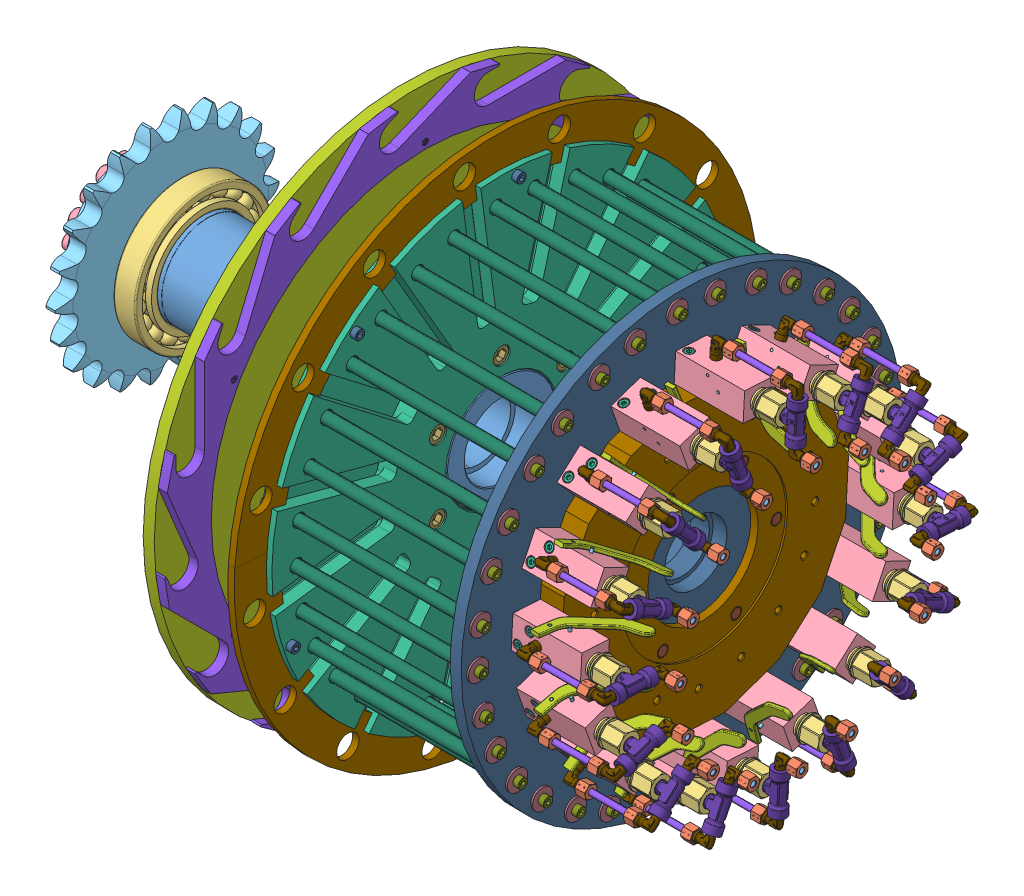
SolidWorks assembly assieme parte rotante, configuration Default. Lengths in mm. (continued)
Components (placement in the parent): (continued)
- AssiemeValvola-7: AssiemeValvola [Default] at (515.3257 -134.8578 488.6421) x (0 0.901303 -0.433189) z (0 -0.433189 -0.901303) size (90.26 138.63 38)
  - RaccordoT-1: RaccordoT [Default] at origin size (43 29.75 16.5)
  - Raccordo a L-1: Raccordo a L [Default] at (-30 0 0) x (0 -1 0) z (0 0 -1) size (28.34 25.51 14.01)
    - 1809_06_10_01-1: 1809_06_10_01 [Default] at origin size (22.49 23 10)
    - 1809_06_10_02-1: 1809_06_10_02 [Default] at origin size (6.5 8.5 8.5)
    - 1809_06_10_03-1: 1809_06_10_03 [Default] at origin size (11.02 15.01 14.01)
  - Raccordo a L-2: Raccordo a L [Default] at (30 0 0) x (0 1 0) z (0 0 -1) size (28.34 25.51 14.01)
    - 1809_06_10_01-1: 1809_06_10_01 [Default] at origin size (22.49 23 10)
    - 1809_06_10_02-1: 1809_06_10_02 [Default] at origin size (6.5 8.5 8.5)
    - 1809_06_10_03-1: 1809_06_10_03 [Default] at origin size (11.02 15.01 14.01)
  - TappoChiusura-1: TappoChiusura [Default] at (0 -32 0) x (0 -1 0) z (0 0 1) size (38.28 26.74 26.74)
  - CorpoValvola-1: CorpoValvola [Default] at (-15 -115.2824 0) size (30 75 34)
  - Raccordo a L-3: Raccordo a L [Default] at (-30 -88.2824 0) x (0 1 0) z (0 0 1) size (28.34 25.51 14.01)
    - 1809_06_10_01-1: 1809_06_10_01 [Default] at origin size (22.49 23 10)
    - 1809_06_10_02-1: 1809_06_10_02 [Default] at origin size (6.5 8.5 8.5)
    - 1809_06_10_03-1: 1809_06_10_03 [Default] at origin size (11.02 15.01 14.01)
  - Spina_3x38-1: Spina_3x38 [Default] at (0 -68.2824 -21) x (-1 0 0) z (0 0 1) size (3 3 38)
  - Spina_3x38-2: Spina_3x38 [Default] at (-10 -80.2824 -21) x (0.996193 0.087174 0) z (0 0 1) size (3 3 38)
  - M5 40mm-3: M5 40mm [ISO 4762 M5 x 40 - 40N] at (-14.6 -108.7824 9) size (45 8.5 8.5)
  - M5 40mm-2: M5 40mm [ISO 4762 M5 x 40 - 40N] at (-14.6 -96.7824 -9) size (45 8.5 8.5)
  - LevaValvola-1: LevaValvola [Default] at (-24.507 -86.571 -17) x (0.996193 0.087174 0) z (0 0 1) size (77.55 60.2 4)
  - Tubo-1: Tubo [Default] at (-30 -15.9665 0) x (1 0 0) z (0 -1 0) size (6 6 56.4)
- AssiemeValvola-8: AssiemeValvola [Default] at (515.3257 -95.0129 541.6718) x (0 0.666921 -0.745128) z (0 -0.745128 -0.666921) size (90.26 138.63 38)
  - RaccordoT-1: RaccordoT [Default] at origin size (43 29.75 16.5)
  - Raccordo a L-1: Raccordo a L [Default] at (-30 0 0) x (0 -1 0) z (0 0 -1) size (28.34 25.51 14.01)
    - 1809_06_10_01-1: 1809_06_10_01 [Default] at origin size (22.49 23 10)
    - 1809_06_10_02-1: 1809_06_10_02 [Default] at origin size (6.5 8.5 8.5)
    - 1809_06_10_03-1: 1809_06_10_03 [Default] at origin size (11.02 15.01 14.01)
  - Raccordo a L-2: Raccordo a L [Default] at (30 0 0) x (0 1 0) z (0 0 -1) size (28.34 25.51 14.01)
    - 1809_06_10_01-1: 1809_06_10_01 [Default] at origin size (22.49 23 10)
    - 1809_06_10_02-1: 1809_06_10_02 [Default] at origin size (6.5 8.5 8.5)
    - 1809_06_10_03-1: 1809_06_10_03 [Default] at origin size (11.02 15.01 14.01)
  - TappoChiusura-1: TappoChiusura [Default] at (0 -32 0) x (0 -1 0) z (0 0 1) size (38.28 26.74 26.74)
  - CorpoValvola-1: CorpoValvola [Default] at (-15 -115.2824 0) size (30 75 34)
  - Raccordo a L-3: Raccordo a L [Default] at (-30 -88.2824 0) x (0 1 0) z (0 0 1) size (28.34 25.51 14.01)
    - 1809_06_10_01-1: 1809_06_10_01 [Default] at origin size (22.49 23 10)
    - 1809_06_10_02-1: 1809_06_10_02 [Default] at origin size (6.5 8.5 8.5)
    - 1809_06_10_03-1: 1809_06_10_03 [Default] at origin size (11.02 15.01 14.01)
  - Spina_3x38-1: Spina_3x38 [Default] at (0 -68.2824 -21) x (-1 0 0) z (0 0 1) size (3 3 38)
  - Spina_3x38-2: Spina_3x38 [Default] at (-10 -80.2824 -21) x (0.996193 0.087174 0) z (0 0 1) size (3 3 38)
  - M5 40mm-3: M5 40mm [ISO 4762 M5 x 40 - 40N] at (-14.6 -108.7824 9) size (45 8.5 8.5)
  - M5 40mm-2: M5 40mm [ISO 4762 M5 x 40 - 40N] at (-14.6 -96.7824 -9) size (45 8.5 8.5)
  - LevaValvola-1: LevaValvola [Default] at (-24.507 -86.571 -17) x (0.996193 0.087174 0) z (0 0 1) size (77.55 60.2 4)
  - Tubo-1: Tubo [Default] at (-30 -15.9665 0) x (1 0 0) z (0 -1 0) size (6 6 56.4)
- AssiemeValvola-9: AssiemeValvola [Default] at (515.3257 -37.9074 575.4168) x (0 0.331007 -0.943628) z (0 -0.943628 -0.331007) size (90.26 138.63 38)
  - RaccordoT-1: RaccordoT [Default] at origin size (43 29.75 16.5)
  - Raccordo a L-1: Raccordo a L [Default] at (-30 0 0) x (0 -1 0) z (0 0 -1) size (28.34 25.51 14.01)
    - 1809_06_10_01-1: 1809_06_10_01 [Default] at origin size (22.49 23 10)
    - 1809_06_10_02-1: 1809_06_10_02 [Default] at origin size (6.5 8.5 8.5)
    - 1809_06_10_03-1: 1809_06_10_03 [Default] at origin size (11.02 15.01 14.01)
  - Raccordo a L-2: Raccordo a L [Default] at (30 0 0) x (0 1 0) z (0 0 -1) size (28.34 25.51 14.01)
    - 1809_06_10_01-1: 1809_06_10_01 [Default] at origin size (22.49 23 10)
    - 1809_06_10_02-1: 1809_06_10_02 [Default] at origin size (6.5 8.5 8.5)
    - 1809_06_10_03-1: 1809_06_10_03 [Default] at origin size (11.02 15.01 14.01)
  - TappoChiusura-1: TappoChiusura [Default] at (0 -32 0) x (0 -1 0) z (0 0 1) size (38.28 26.74 26.74)
  - CorpoValvola-1: CorpoValvola [Default] at (-15 -115.2824 0) size (30 75 34)
  - Raccordo a L-3: Raccordo a L [Default] at (-30 -88.2824 0) x (0 1 0) z (0 0 1) size (28.34 25.51 14.01)
    - 1809_06_10_01-1: 1809_06_10_01 [Default] at origin size (22.49 23 10)
    - 1809_06_10_02-1: 1809_06_10_02 [Default] at origin size (6.5 8.5 8.5)
    - 1809_06_10_03-1: 1809_06_10_03 [Default] at origin size (11.02 15.01 14.01)
  - Spina_3x38-1: Spina_3x38 [Default] at (0 -68.2824 -21) x (-1 0 0) z (0 0 1) size (3 3 38)
  - Spina_3x38-2: Spina_3x38 [Default] at (-10 -80.2824 -21) x (0.996193 0.087174 0) z (0 0 1) size (3 3 38)
  - M5 40mm-3: M5 40mm [ISO 4762 M5 x 40 - 40N] at (-14.6 -108.7824 9) size (45 8.5 8.5)
  - M5 40mm-2: M5 40mm [ISO 4762 M5 x 40 - 40N] at (-14.6 -96.7824 -9) size (45 8.5 8.5)
  - LevaValvola-1: LevaValvola [Default] at (-24.507 -86.571 -17) x (0.996193 0.087174 0) z (0 0 1) size (77.55 60.2 4)
  - Tubo-1: Tubo [Default] at (-30 -15.9665 0) x (1 0 0) z (0 -1 0) size (6 6 56.4)
- AssiemeValvola-10: AssiemeValvola [Default] at (515.3257 27.7648 584.7399) x (0 -0.055301 -0.99847) z (0 -0.99847 0.055301) size (90.26 138.63 38)
  - RaccordoT-1: RaccordoT [Default] at origin size (43 29.75 16.5)
  - Raccordo a L-1: Raccordo a L [Default] at (-30 0 0) x (0 -1 0) z (0 0 -1) size (28.34 25.51 14.01)
    - 1809_06_10_01-1: 1809_06_10_01 [Default] at origin size (22.49 23 10)
    - 1809_06_10_02-1: 1809_06_10_02 [Default] at origin size (6.5 8.5 8.5)
    - 1809_06_10_03-1: 1809_06_10_03 [Default] at origin size (11.02 15.01 14.01)
  - Raccordo a L-2: Raccordo a L [Default] at (30 0 0) x (0 1 0) z (0 0 -1) size (28.34 25.51 14.01)
    - 1809_06_10_01-1: 1809_06_10_01 [Default] at origin size (22.49 23 10)
    - 1809_06_10_02-1: 1809_06_10_02 [Default] at origin size (6.5 8.5 8.5)
    - 1809_06_10_03-1: 1809_06_10_03 [Default] at origin size (11.02 15.01 14.01)
  - TappoChiusura-1: TappoChiusura [Default] at (0 -32 0) x (0 -1 0) z (0 0 1) size (38.28 26.74 26.74)
  - CorpoValvola-1: CorpoValvola [Default] at (-15 -115.2824 0) size (30 75 34)
  - Raccordo a L-3: Raccordo a L [Default] at (-30 -88.2824 0) x (0 1 0) z (0 0 1) size (28.34 25.51 14.01)
    - 1809_06_10_01-1: 1809_06_10_01 [Default] at origin size (22.49 23 10)
    - 1809_06_10_02-1: 1809_06_10_02 [Default] at origin size (6.5 8.5 8.5)
    - 1809_06_10_03-1: 1809_06_10_03 [Default] at origin size (11.02 15.01 14.01)
  - Spina_3x38-1: Spina_3x38 [Default] at (0 -68.2824 -21) x (-1 0 0) z (0 0 1) size (3 3 38)
  - Spina_3x38-2: Spina_3x38 [Default] at (-10 -80.2824 -21) x (0.996193 0.087174 0) z (0 0 1) size (3 3 38)
  - M5 40mm-3: M5 40mm [ISO 4762 M5 x 40 - 40N] at (-14.6 -108.7824 9) size (45 8.5 8.5)
  - M5 40mm-2: M5 40mm [ISO 4762 M5 x 40 - 40N] at (-14.6 -96.7824 -9) size (45 8.5 8.5)
  - LevaValvola-1: LevaValvola [Default] at (-24.507 -86.571 -17) x (0.996193 0.087174 0) z (0 0 1) size (77.55 60.2 4)
  - Tubo-1: Tubo [Default] at (-30 -15.9665 0) x (1 0 0) z (0 -1 0) size (6 6 56.4)
- AssiemeValvola-11: AssiemeValvola [Default] at (515.3257 92.0058 568.2215) x (0 -0.433189 -0.901303) z (0 -0.901303 0.433189) size (90.26 138.63 38)
  - RaccordoT-1: RaccordoT [Default] at origin size (43 29.75 16.5)
  - Raccordo a L-1: Raccordo a L [Default] at (-30 0 0) x (0 -1 0) z (0 0 -1) size (28.34 25.51 14.01)
    - 1809_06_10_01-1: 1809_06_10_01 [Default] at origin size (22.49 23 10)
    - 1809_06_10_02-1: 1809_06_10_02 [Default] at origin size (6.5 8.5 8.5)
    - 1809_06_10_03-1: 1809_06_10_03 [Default] at origin size (11.02 15.01 14.01)
  - Raccordo a L-2: Raccordo a L [Default] at (30 0 0) x (0 1 0) z (0 0 -1) size (28.34 25.51 14.01)
    - 1809_06_10_01-1: 1809_06_10_01 [Default] at origin size (22.49 23 10)
    - 1809_06_10_02-1: 1809_06_10_02 [Default] at origin size (6.5 8.5 8.5)
    - 1809_06_10_03-1: 1809_06_10_03 [Default] at origin size (11.02 15.01 14.01)
  - TappoChiusura-1: TappoChiusura [Default] at (0 -32 0) x (0 -1 0) z (0 0 1) size (38.28 26.74 26.74)
  - CorpoValvola-1: CorpoValvola [Default] at (-15 -115.2824 0) size (30 75 34)
  - Raccordo a L-3: Raccordo a L [Default] at (-30 -88.2824 0) x (0 1 0) z (0 0 1) size (28.34 25.51 14.01)
    - 1809_06_10_01-1: 1809_06_10_01 [Default] at origin size (22.49 23 10)
    - 1809_06_10_02-1: 1809_06_10_02 [Default] at origin size (6.5 8.5 8.5)
    - 1809_06_10_03-1: 1809_06_10_03 [Default] at origin size (11.02 15.01 14.01)
  - Spina_3x38-1: Spina_3x38 [Default] at (0 -68.2824 -21) x (-1 0 0) z (0 0 1) size (3 3 38)
  - Spina_3x38-2: Spina_3x38 [Default] at (-10 -80.2824 -21) x (0.996193 0.087174 0) z (0 0 1) size (3 3 38)
  - M5 40mm-3: M5 40mm [ISO 4762 M5 x 40 - 40N] at (-14.6 -108.7824 9) size (45 8.5 8.5)
  - M5 40mm-2: M5 40mm [ISO 4762 M5 x 40 - 40N] at (-14.6 -96.7824 -9) size (45 8.5 8.5)
  - LevaValvola-1: LevaValvola [Default] at (-24.507 -86.571 -17) x (0.996193 0.087174 0) z (0 0 1) size (77.55 60.2 4)
  - Tubo-1: Tubo [Default] at (-30 -15.9665 0) x (1 0 0) z (0 -1 0) size (6 6 56.4)
- AssiemeValvola-12: AssiemeValvola [Default] at (515.3257 145.0355 528.3766) x (0 -0.745128 -0.666921) z (0 -0.666921 0.745128) size (90.26 138.63 38)
  - RaccordoT-1: RaccordoT [Default] at origin size (43 29.75 16.5)
  - Raccordo a L-1: Raccordo a L [Default] at (-30 0 0) x (0 -1 0) z (0 0 -1) size (28.34 25.51 14.01)
    - 1809_06_10_01-1: 1809_06_10_01 [Default] at origin size (22.49 23 10)
    - 1809_06_10_02-1: 1809_06_10_02 [Default] at origin size (6.5 8.5 8.5)
    - 1809_06_10_03-1: 1809_06_10_03 [Default] at origin size (11.02 15.01 14.01)
  - Raccordo a L-2: Raccordo a L [Default] at (30 0 0) x (0 1 0) z (0 0 -1) size (28.34 25.51 14.01)
    - 1809_06_10_01-1: 1809_06_10_01 [Default] at origin size (22.49 23 10)
    - 1809_06_10_02-1: 1809_06_10_02 [Default] at origin size (6.5 8.5 8.5)
    - 1809_06_10_03-1: 1809_06_10_03 [Default] at origin size (11.02 15.01 14.01)
  - TappoChiusura-1: TappoChiusura [Default] at (0 -32 0) x (0 -1 0) z (0 0 1) size (38.28 26.74 26.74)
  - CorpoValvola-1: CorpoValvola [Default] at (-15 -115.2824 0) size (30 75 34)
  - Raccordo a L-3: Raccordo a L [Default] at (-30 -88.2824 0) x (0 1 0) z (0 0 1) size (28.34 25.51 14.01)
    - 1809_06_10_01-1: 1809_06_10_01 [Default] at origin size (22.49 23 10)
    - 1809_06_10_02-1: 1809_06_10_02 [Default] at origin size (6.5 8.5 8.5)
    - 1809_06_10_03-1: 1809_06_10_03 [Default] at origin size (11.02 15.01 14.01)
  - Spina_3x38-1: Spina_3x38 [Default] at (0 -68.2824 -21) x (-1 0 0) z (0 0 1) size (3 3 38)
  - Spina_3x38-2: Spina_3x38 [Default] at (-10 -80.2824 -21) x (0.996193 0.087174 0) z (0 0 1) size (3 3 38)
  - M5 40mm-3: M5 40mm [ISO 4762 M5 x 40 - 40N] at (-14.6 -108.7824 9) size (45 8.5 8.5)
  - M5 40mm-2: M5 40mm [ISO 4762 M5 x 40 - 40N] at (-14.6 -96.7824 -9) size (45 8.5 8.5)
  - LevaValvola-1: LevaValvola [Default] at (-24.507 -86.571 -17) x (0.996193 0.087174 0) z (0 0 1) size (77.55 60.2 4)
  - Tubo-1: Tubo [Default] at (-30 -15.9665 0) x (1 0 0) z (0 -1 0) size (6 6 56.4)
- AssiemeValvola-13: AssiemeValvola [Default] at (515.3257 178.7805 471.2711) x (0 -0.943628 -0.331007) z (0 -0.331007 0.943628) size (90.26 138.63 38)
  - RaccordoT-1: RaccordoT [Default] at origin size (43 29.75 16.5)
  - Raccordo a L-1: Raccordo a L [Default] at (-30 0 0) x (0 -1 0) z (0 0 -1) size (28.34 25.51 14.01)
    - 1809_06_10_01-1: 1809_06_10_01 [Default] at origin size (22.49 23 10)
    - 1809_06_10_02-1: 1809_06_10_02 [Default] at origin size (6.5 8.5 8.5)
    - 1809_06_10_03-1: 1809_06_10_03 [Default] at origin size (11.02 15.01 14.01)
  - Raccordo a L-2: Raccordo a L [Default] at (30 0 0) x (0 1 0) z (0 0 -1) size (28.34 25.51 14.01)
    - 1809_06_10_01-1: 1809_06_10_01 [Default] at origin size (22.49 23 10)
    - 1809_06_10_02-1: 1809_06_10_02 [Default] at origin size (6.5 8.5 8.5)
    - 1809_06_10_03-1: 1809_06_10_03 [Default] at origin size (11.02 15.01 14.01)
  - TappoChiusura-1: TappoChiusura [Default] at (0 -32 0) x (0 -1 0) z (0 0 1) size (38.28 26.74 26.74)
  - CorpoValvola-1: CorpoValvola [Default] at (-15 -115.2824 0) size (30 75 34)
  - Raccordo a L-3: Raccordo a L [Default] at (-30 -88.2824 0) x (0 1 0) z (0 0 1) size (28.34 25.51 14.01)
    - 1809_06_10_01-1: 1809_06_10_01 [Default] at origin size (22.49 23 10)
    - 1809_06_10_02-1: 1809_06_10_02 [Default] at origin size (6.5 8.5 8.5)
    - 1809_06_10_03-1: 1809_06_10_03 [Default] at origin size (11.02 15.01 14.01)
  - Spina_3x38-1: Spina_3x38 [Default] at (0 -68.2824 -21) x (-1 0 0) z (0 0 1) size (3 3 38)
  - Spina_3x38-2: Spina_3x38 [Default] at (-10 -80.2824 -21) x (0.996193 0.087174 0) z (0 0 1) size (3 3 38)
  - M5 40mm-3: M5 40mm [ISO 4762 M5 x 40 - 40N] at (-14.6 -108.7824 9) size (45 8.5 8.5)
  - M5 40mm-2: M5 40mm [ISO 4762 M5 x 40 - 40N] at (-14.6 -96.7824 -9) size (45 8.5 8.5)
  - LevaValvola-1: LevaValvola [Default] at (-24.507 -86.571 -17) x (0.996193 0.087174 0) z (0 0 1) size (77.55 60.2 4)
  - Tubo-1: Tubo [Default] at (-30 -15.9665 0) x (1 0 0) z (0 -1 0) size (6 6 56.4)
- AssiemeValvola-14: AssiemeValvola [Default] at (515.3257 188.1036 405.5989) x (0 -0.99847 0.055301) z (0 0.055301 0.99847) size (90.26 138.63 38)
  - RaccordoT-1: RaccordoT [Default] at origin size (43 29.75 16.5)
  - Raccordo a L-1: Raccordo a L [Default] at (-30 0 0) x (0 -1 0) z (0 0 -1) size (28.34 25.51 14.01)
    - 1809_06_10_01-1: 1809_06_10_01 [Default] at origin size (22.49 23 10)
    - 1809_06_10_02-1: 1809_06_10_02 [Default] at origin size (6.5 8.5 8.5)
    - 1809_06_10_03-1: 1809_06_10_03 [Default] at origin size (11.02 15.01 14.01)
  - Raccordo a L-2: Raccordo a L [Default] at (30 0 0) x (0 1 0) z (0 0 -1) size (28.34 25.51 14.01)
    - 1809_06_10_01-1: 1809_06_10_01 [Default] at origin size (22.49 23 10)
    - 1809_06_10_02-1: 1809_06_10_02 [Default] at origin size (6.5 8.5 8.5)
    - 1809_06_10_03-1: 1809_06_10_03 [Default] at origin size (11.02 15.01 14.01)
  - TappoChiusura-1: TappoChiusura [Default] at (0 -32 0) x (0 -1 0) z (0 0 1) size (38.28 26.74 26.74)
  - CorpoValvola-1: CorpoValvola [Default] at (-15 -115.2824 0) size (30 75 34)
  - Raccordo a L-3: Raccordo a L [Default] at (-30 -88.2824 0) x (0 1 0) z (0 0 1) size (28.34 25.51 14.01)
    - 1809_06_10_01-1: 1809_06_10_01 [Default] at origin size (22.49 23 10)
    - 1809_06_10_02-1: 1809_06_10_02 [Default] at origin size (6.5 8.5 8.5)
    - 1809_06_10_03-1: 1809_06_10_03 [Default] at origin size (11.02 15.01 14.01)
  - Spina_3x38-1: Spina_3x38 [Default] at (0 -68.2824 -21) x (-1 0 0) z (0 0 1) size (3 3 38)
  - Spina_3x38-2: Spina_3x38 [Default] at (-10 -80.2824 -21) x (0.996193 0.087174 0) z (0 0 1) size (3 3 38)
  - M5 40mm-3: M5 40mm [ISO 4762 M5 x 40 - 40N] at (-14.6 -108.7824 9) size (45 8.5 8.5)
  - M5 40mm-2: M5 40mm [ISO 4762 M5 x 40 - 40N] at (-14.6 -96.7824 -9) size (45 8.5 8.5)
  - LevaValvola-1: LevaValvola [Default] at (-24.507 -86.571 -17) x (0.996193 0.087174 0) z (0 0 1) size (77.55 60.2 4)
  - Tubo-1: Tubo [Default] at (-30 -15.9665 0) x (1 0 0) z (0 -1 0) size (6 6 56.4)
- AssiemeValvola-15: AssiemeValvola [Default] at (515.3257 171.5852 341.3579) x (0 -0.901303 0.433189) z (0 0.433189 0.901303) size (90.26 138.63 38)
  - RaccordoT-1: RaccordoT [Default] at origin size (43 29.75 16.5)
  - Raccordo a L-1: Raccordo a L [Default] at (-30 0 0) x (0 -1 0) z (0 0 -1) size (28.34 25.51 14.01)
    - 1809_06_10_01-1: 1809_06_10_01 [Default] at origin size (22.49 23 10)
    - 1809_06_10_02-1: 1809_06_10_02 [Default] at origin size (6.5 8.5 8.5)
    - 1809_06_10_03-1: 1809_06_10_03 [Default] at origin size (11.02 15.01 14.01)
  - Raccordo a L-2: Raccordo a L [Default] at (30 0 0) x (0 1 0) z (0 0 -1) size (28.34 25.51 14.01)
    - 1809_06_10_01-1: 1809_06_10_01 [Default] at origin size (22.49 23 10)
    - 1809_06_10_02-1: 1809_06_10_02 [Default] at origin size (6.5 8.5 8.5)
    - 1809_06_10_03-1: 1809_06_10_03 [Default] at origin size (11.02 15.01 14.01)
  - TappoChiusura-1: TappoChiusura [Default] at (0 -32 0) x (0 -1 0) z (0 0 1) size (38.28 26.74 26.74)
  - CorpoValvola-1: CorpoValvola [Default] at (-15 -115.2824 0) size (30 75 34)
  - Raccordo a L-3: Raccordo a L [Default] at (-30 -88.2824 0) x (0 1 0) z (0 0 1) size (28.34 25.51 14.01)
    - 1809_06_10_01-1: 1809_06_10_01 [Default] at origin size (22.49 23 10)
    - 1809_06_10_02-1: 1809_06_10_02 [Default] at origin size (6.5 8.5 8.5)
    - 1809_06_10_03-1: 1809_06_10_03 [Default] at origin size (11.02 15.01 14.01)
  - Spina_3x38-1: Spina_3x38 [Default] at (0 -68.2824 -21) x (-1 0 0) z (0 0 1) size (3 3 38)
  - Spina_3x38-2: Spina_3x38 [Default] at (-10 -80.2824 -21) x (0.996193 0.087174 0) z (0 0 1) size (3 3 38)
  - M5 40mm-3: M5 40mm [ISO 4762 M5 x 40 - 40N] at (-14.6 -108.7824 9) size (45 8.5 8.5)
  - M5 40mm-2: M5 40mm [ISO 4762 M5 x 40 - 40N] at (-14.6 -96.7824 -9) size (45 8.5 8.5)
  - LevaValvola-1: LevaValvola [Default] at (-24.507 -86.571 -17) x (0.996193 0.087174 0) z (0 0 1) size (77.55 60.2 4)
  - Tubo-1: Tubo [Default] at (-30 -15.9665 0) x (1 0 0) z (0 -1 0) size (6 6 56.4)
- AssiemeValvola-16: AssiemeValvola [Default] at (515.3257 131.7403 288.3282) x (0 -0.666921 0.745128) z (0 0.745128 0.666921) size (90.26 138.63 38)
  - RaccordoT-1: RaccordoT [Default] at origin size (43 29.75 16.5)
  - Raccordo a L-1: Raccordo a L [Default] at (-30 0 0) x (0 -1 0) z (0 0 -1) size (28.34 25.51 14.01)
    - 1809_06_10_01-1: 1809_06_10_01 [Default] at origin size (22.49 23 10)
    - 1809_06_10_02-1: 1809_06_10_02 [Default] at origin size (6.5 8.5 8.5)
    - 1809_06_10_03-1: 1809_06_10_03 [Default] at origin size (11.02 15.01 14.01)
  - Raccordo a L-2: Raccordo a L [Default] at (30 0 0) x (0 1 0) z (0 0 -1) size (28.34 25.51 14.01)
    - 1809_06_10_01-1: 1809_06_10_01 [Default] at origin size (22.49 23 10)
    - 1809_06_10_02-1: 1809_06_10_02 [Default] at origin size (6.5 8.5 8.5)
    - 1809_06_10_03-1: 1809_06_10_03 [Default] at origin size (11.02 15.01 14.01)
  - TappoChiusura-1: TappoChiusura [Default] at (0 -32 0) x (0 -1 0) z (0 0 1) size (38.28 26.74 26.74)
  - CorpoValvola-1: CorpoValvola [Default] at (-15 -115.2824 0) size (30 75 34)
  - Raccordo a L-3: Raccordo a L [Default] at (-30 -88.2824 0) x (0 1 0) z (0 0 1) size (28.34 25.51 14.01)
    - 1809_06_10_01-1: 1809_06_10_01 [Default] at origin size (22.49 23 10)
    - 1809_06_10_02-1: 1809_06_10_02 [Default] at origin size (6.5 8.5 8.5)
    - 1809_06_10_03-1: 1809_06_10_03 [Default] at origin size (11.02 15.01 14.01)
  - Spina_3x38-1: Spina_3x38 [Default] at (0 -68.2824 -21) x (-1 0 0) z (0 0 1) size (3 3 38)
  - Spina_3x38-2: Spina_3x38 [Default] at (-10 -80.2824 -21) x (0.996193 0.087174 0) z (0 0 1) size (3 3 38)
  - M5 40mm-3: M5 40mm [ISO 4762 M5 x 40 - 40N] at (-14.6 -108.7824 9) size (45 8.5 8.5)
  - M5 40mm-2: M5 40mm [ISO 4762 M5 x 40 - 40N] at (-14.6 -96.7824 -9) size (45 8.5 8.5)
  - LevaValvola-1: LevaValvola [Default] at (-24.507 -86.571 -17) x (0.996193 0.087174 0) z (0 0 1) size (77.55 60.2 4)
  - Tubo-1: Tubo [Default] at (-30 -15.9665 0) x (1 0 0) z (0 -1 0) size (6 6 56.4)
- Disco alimentazione guarnizione fi24.4-1: Disco alimentazione guarnizione fi24.4 [Default] at (198.0433 18.3637 415) x (0 0.065403 0.997859) z (-1 0 0) size (570 285 7.35)
- Disco alimentazione guarnizione fi24.4-2: Disco alimentazione guarnizione fi24.4 [Default] at (198.0433 18.3637 415) x (0 -0.065403 -0.997859) z (-1 0 0) size (570 285 7.35)
- m6 12mm-1: m6 12mm [ISO 4762 M6 x 12 - 12N] at (210.0433 200.6849 574.8914) x (-1 0 0) z (0 0.793353 -0.608761) size (18 10 10)
- m6 12mm-7: m6 12mm [ISO 4762 M6 x 12 - 12N] at (210.0433 260.3445 399.1397) x (-1 0 0) z (0 0.793353 -0.608761) size (18 10 10)
- m6 12mm-8: m6 12mm [ISO 4762 M6 x 12 - 12N] at (210.0433 96.3128 185.3694) x (-1 0 0) z (0 0.793353 -0.608761) size (18 10 10)
- m6 12mm-9: m6 12mm [ISO 4762 M6 x 12 - 12N] at (210.0433 -59.5854 644.6306) x (-1 0 0) z (0 -0.793353 -0.608761) size (18 10 10)
- m6 12mm-10: m6 12mm [ISO 4762 M6 x 12 - 12N] at (210.0433 -223.6171 430.8603) x (-1 0 0) z (0 -0.793353 -0.608761) size (18 10 10)
- m6 12mm-11: m6 12mm [ISO 4762 M6 x 12 - 12N] at (210.0433 -163.9575 255.1086) x (-1 0 0) z (0 0.793353 -0.608761) size (18 10 10)
Mates (geometry in assembly coordinates):
- Concentrico1: concentric anti-aligned: circle of albero rotazione piatti-1; circle of seger 100mm-1
- Coincidente1: coincident anti-aligned: plane of albero rotazione piatti-1 through (-143.4567 18.3637 415) normal (-1 0 0); plane of seger 100mm-1 through (-143.4567 18.3637 415) normal (1 0 0)
- Coincidente2: coincident aligned: plane of albero rotazione piatti-1 through (60.413 18.3637 415) normal (0 1 0); plane of seger 100mm-1 through (-146.4567 18.3637 415) normal (0 1 0)
- Concentrico21: concentric aligned: cylinder of albero rotazione piatti-1 through (60.413 18.3637 415) axis (1 0 0) radius 50; cylinder of SKF - 6020 - 20,DE,NC,20_68-1 through (-152.0942 18.3637 415) axis (1 0 0) radius 50
- Coincidente3: coincident anti-aligned: plane of seger 100mm-1 through (-143.4567 18.3637 415) normal (1 0 0); plane of SKF - 6020 - 20,DE,NC,20_68-1 through (-143.4567 -33.4256 439.9823) normal (-1 0 0)
- Concentrico3: concentric aligned: cylinder of albero rotazione piatti-1 through (60.413 18.3637 415) axis (1 0 0) radius 47.5; cylinder of calettatore d95-1 through (-199.9572 18.3637 415) axis (1 0 0) radius 47.5
- Concentrico4: concentric anti-aligned: cylinder of calettatore d95-1 through (-196.9572 18.3637 415) axis (1 0 0) radius 67.5; cylinder of pulegia z =50-1 through (-170.9572 18.3637 415) axis (-1 0 0) radius 67.5
- Coincidente4: coincident anti-aligned: plane of calettatore d95-1 through (-170.9572 84.9137 415) normal (1 0 0); plane of pulegia z =50-1 through (-170.9572 18.3637 415) normal (-1 0 0)
- Coincidente5: coincident anti-aligned: plane of albero rotazione piatti-1 through (-155.9567 18.3637 415) normal (-1 0 0); plane of pulegia z =50-1 through (-155.9567 18.3637 415) normal (1 0 0)
- Coincidente6: coincident aligned: plane of calettatore d95-1 through (-184.9572 18.3637 415) normal (0 1 0); plane of pulegia z =50-1 through (-173.9167 18.3637 415) normal (0 1 0)
- Coincidente7: coincident aligned: plane of albero rotazione piatti-1 through (60.413 18.3637 415) normal (0 1 0); plane of calettatore d95-1 through (-184.9572 18.3637 415) normal (0 1 0)
- Concentrico5: concentric aligned: cylinder of albero rotazione piatti-1 through (60.413 18.3637 415) axis (1 0 0) radius 49.75; cylinder of SKF - 6020 - 20,DE,NC,20_68-2 through (41.4058 18.3637 415) axis (1 0 0) radius 50
- Coincidente8: coincident anti-aligned: plane of albero rotazione piatti-1 through (74.0433 18.3637 415) normal (-1 0 0); plane of SKF - 6020 - 20,DE,NC,20_68-2 through (74.0433 -28.0673 437.2803) normal (1 0 0)
- Concentrico6: concentric aligned: cylinder of albero rotazione piatti-1 through (60.413 18.3637 415) axis (1 0 0) radius 60; cylinder of Disco supporto montaggio e Colonne-1 through (5.3377 18.3637 415) axis (1 0 0) radius 60
- Concentrico7: concentric aligned: cylinder of albero rotazione piatti-1 through (101.3656 98.3637 415) axis (1 0 0) radius 6.25; cylinder of Disco supporto montaggio e Colonne-1 through (204.0433 98.3637 415) axis (1 0 0) radius 9.25
- Coincidente9: coincident anti-aligned: plane of albero rotazione piatti-1 through (175.0433 18.3637 415) normal (1 0 0); plane of Disco supporto montaggio e Colonne-1 through (175.0433 18.3637 415) normal (-1 0 0)
- Concentrico8: concentric anti-aligned: cylinder of albero rotazione piatti-1 through (60.413 18.3637 415) axis (1 0 0) radius 60; cylinder of piatto rotante porta tappi-1 through (111.0433 18.3637 415) axis (-1 0 0) radius 60
- Concentrico9: concentric aligned: circle of albero rotazione piatti-1; circle of piatto rotante porta tappi-1
- Coincidente10: coincident anti-aligned: plane of albero rotazione piatti-1 through (119.0433 18.3637 415) normal (-1 0 0); plane of piatto rotante porta tappi-1 through (119.0433 18.3637 415) normal (1 0 0)
- Concentrico10: concentric aligned: cylinder of piatto rotante porta tappi-1 through (119.0433 18.3637 415) axis (-1 0 0) radius 233; cylinder of disco trasportatore tappi 31-1 through (121.0433 18.3637 415) axis (-1 0 0) radius 233
- Tangente2: tangent: cylinder of piatto rotante porta tappi-1 through (98.5243 -101.6363 622.8461) axis (1 0 0) radius 3.25; curve of disco trasportatore tappi 31-1
- Coincidente13: coincident anti-aligned: plane of piatto rotante porta tappi-1 through (111.0433 18.3637 415) normal (1 0 0); plane of disco trasportatore tappi 31-1 through (111.0433 18.3637 415) normal (-1 0 0)
- Concentrico11: concentric anti-aligned: cylinder of albero rotazione piatti-1 through (60.413 18.3637 415) axis (1 0 0) radius 40; cylinder of disco trascinato porta distributore vuoto-1 through (400.0433 18.3637 415) axis (-1 0 0) radius 30
- Concentrico12: concentric anti-aligned: cylinder of Disco supporto montaggio e Colonne-1 through (204.0433 -202.0247 450.2415) axis (1 0 0) radius 6; cylinder of disco trascinato porta distributore vuoto-1 through (417.0139 -202.0247 450.2415) axis (-1 0 0) radius 6
- Coincidente14: coincident anti-aligned: plane of Distributore Rotante-1 through (400.0433 18.3637 415) normal (-1 0 0); plane of disco trascinato porta distributore vuoto-1 through (400.0433 18.3637 415) normal (1 0 0)
- Concentrico13: concentric anti-aligned: circle of Distributore Rotante-1; circle of disco trascinato porta distributore vuoto-1
- Concentrico14: concentric anti-aligned: cylinder of Distributore Rotante-1 through (230.3377 18.3637 415) axis (1 0 0) radius 60; cylinder of disco trascinato porta distributore vuoto-1 through (415.0433 18.3637 415) axis (-1 0 0) radius 67.5
- Concentrico15: concentric anti-aligned: cylinder of disco trascinato porta distributore vuoto-1 through (388.0433 -53.0243 378.8925) axis (1 0 0) radius 6.25; cylinder of m12 35mm-1 through (344.2933 -53.0243 378.8925) axis (-1 0 0) radius 6
- Coincidente15: coincident anti-aligned: plane of disco trascinato porta distributore vuoto-1 through (388.0433 18.3637 415) normal (-1 0 0); plane of m12 35mm-1 through (388.0433 -45.2301 383.3925) normal (1 0 0)
- Parallelo1: parallel anti-aligned: plane of m12 35mm-1 through (382.0433 -47.9668 381.8125) normal (0 -1 0)
- Concentrico16: concentric aligned: cylinder of Disco supporto montaggio e Colonne-1 through (204.0433 -21.6363 345.718) axis (1 0 0) radius 9.25; cylinder of m12 90mm-3 through (234.7933 -21.6363 345.718) axis (1 0 0) radius 6
- Coincidente17: coincident anti-aligned: plane of Disco supporto montaggio e Colonne-1 through (191.0433 -27.049 342.593) normal (1 0 0); plane of m12 90mm-3 through (191.0433 -29.4305 341.218) normal (-1 0 0)
- Parallelo2: parallel aligned: plane of m12 35mm-1 through (382.0433 -47.9668 381.8125) normal (0 -1 0); plane of m12 90mm-3 through (197.0433 -16.5788 348.6379) normal (0 -1 0)
- Concentrico171: concentric anti-aligned: cylinder of piatto rotante porta tappi-1 through (98.5243 -101.6363 207.1539) axis (1 0 0) radius 3.25; cylinder of rondella m6 22mm-1 through (64.1183 -101.6363 207.1539) axis (-1 0 0) radius 3.3
- Coincidente191: coincident anti-aligned: plane of piatto rotante porta tappi-1 through (99.0433 18.3637 415) normal (-1 0 0); plane of rondella m6 22mm-1 through (99.0433 -101.6363 210.4539) normal (1 0 0)
- Parallelo3: parallel anti-aligned: plane of rondella m6 22mm-1 through (99.0433 -101.6363 207.1539) normal (0 -1 0)
- Concentrico181: concentric aligned: cylinder of rondella m6 22mm-1 through (64.1183 -101.6363 207.1539) axis (-1 0 0) radius 3.3; cylinder of M6 20mm-1 through (59.2933 -101.6363 207.1539) axis (-1 0 0) radius 5
- Coincidente211: coincident anti-aligned: plane of rondella m6 22mm-1 through (97.0433 -101.6363 218.1539) normal (-1 0 0); plane of M6 20mm-1 through (97.0433 -97.3062 204.6539) normal (1 0 0)
- Parallelo4: parallel aligned: plane of m12 35mm-1 through (382.0433 -47.9668 381.8125) normal (0 -0.5 -0.866025); plane of M6 20mm-1 through (94.0433 -101.6363 210.0892) normal (0 -0.5 -0.866025)
- Concentrico19: concentric anti-aligned: cylinder of Disco supporto montaggio e Colonne-1 through (204.0433 70.1437 197.9013) axis (1 0 0) radius 6; cylinder of asta scorrimento carello-1 through (400.0433 70.1437 197.9013) axis (-1 0 0) radius 6
- Concentrico201: concentric aligned: cylinder of asta scorrimento carello-1 through (175.0433 70.1437 197.9013) axis (-1 0 0) radius 3.2; cylinder of rondella m6 22mm-7 through (140.1183 70.1437 197.9013) axis (-1 0 0) radius 3.3
- Coincidente231: coincident anti-aligned: plane of asta scorrimento carello-1 through (175.0433 70.1437 197.9013) normal (-1 0 0); plane of rondella m6 22mm-7 through (175.0433 70.1437 201.2013) normal (1 0 0)
- Concentrico211: concentric aligned: cylinder of rondella m6 22mm-7 through (140.1183 70.1437 197.9013) axis (-1 0 0) radius 3.3; cylinder of M6 16mm-1 through (135.2933 70.1437 197.9013) axis (-1 0 0) radius 5
- Coincidente241: coincident anti-aligned: plane of rondella m6 22mm-7 through (173.0433 70.1437 208.9013) normal (-1 0 0); plane of M6 16mm-1 through (173.0433 75.1437 197.9013) normal (1 0 0)
- Parallelo5: parallel aligned: plane of asta scorrimento carello-1 through (287.5433 70.1437 197.9013) normal (0 0 -1); plane of M6 16mm-1 through (170.0433 68.6761 200.4433) normal (0 0 -1)
- Parallelo9: parallel anti-aligned: plane of rondella m6 22mm-7 through (175.0433 70.1437 197.9013) normal (0 0 1); plane of M6 16mm-1 through (170.0433 68.6761 200.4433) normal (0 0 -1)
- Coincidente30: coincident anti-aligned: plane of Disco supporto montaggio e Colonne-1 through (175.0433 18.3637 415) normal (-1 0 0); plane of rondella m6 22mm-7 through (175.0433 70.1437 201.2013) normal (1 0 0)
- Coincidente31: coincident anti-aligned: plane of disco trascinato porta distributore vuoto-1 through (400.0433 18.3637 415) normal (1 0 0); plane of rondella m6 22mm-8 through (400.0433 70.1437 201.2013) normal (-1 0 0)
- Coincidente32: coincident anti-aligned: plane of Distributore Rotante-1 through (400.0433 40.5763 258.5322) normal (0 0.331007 -0.943628); plane of AssiemeValvola-1/CorpoValvola-1 through (400.0433 85.7114 274.3647) normal (0 -0.331007 0.943628)
- Coincidente33: coincident anti-aligned: plane of disco trascinato porta distributore vuoto-1 through (400.0433 18.3637 415) normal (1 0 0); plane of AssiemeValvola-1/CorpoValvola-1 through (400.0433 95.6416 246.0559) normal (-1 0 0)
- Concentrico22: concentric anti-aligned: cylinder of Distributore Rotante-1 through (412.5433 55.4365 309.3136) axis (0 0.331007 -0.943628) radius 3; cylinder of AssiemeValvola-1/CorpoValvola-1 through (412.5433 69.6697 268.7376) axis (0 -0.331007 0.943628) radius 3
- Concentrico23: concentric anti-aligned: cylinder of Disco supporto montaggio e Colonne-1 through (198.0433 18.3637 415) axis (-1 0 0) radius 235; cylinder of Disco alimentazione guarnizione fi24.4-2 through (191.0433 18.3637 415) axis (1 0 0) radius 235
- Concentrico24: concentric anti-aligned: cylinder of Disco supporto montaggio e Colonne-1 through (198.0433 18.3637 415) axis (-1 0 0) radius 235; cylinder of Disco alimentazione guarnizione fi24.4-1 through (191.0433 18.3637 415) axis (1 0 0) radius 235
- Coincidente34: coincident anti-aligned: plane of Disco alimentazione guarnizione fi24.4-1 through (191.0433 33.7334 649.4968) normal (0 -0.997859 0.065403); plane of Disco alimentazione guarnizione fi24.4-2 through (191.0433 37.0036 699.3898) normal (0 0.997859 -0.065403)
- Coincidente35: coincident aligned: plane of Disco alimentazione guarnizione fi24.4-1 through (198.0433 18.3637 415) normal (1 0 0); plane of Disco alimentazione guarnizione fi24.4-2 through (198.0433 18.3637 415) normal (1 0 0)
- Concentrico25: concentric anti-aligned: cylinder of Disco supporto montaggio e Colonne-1 through (188.8509 -59.5854 644.6306) axis (1 0 0) radius 3.25; circle of Disco alimentazione guarnizione fi24.4-2
- Coincidente36: coincident anti-aligned: plane of Disco supporto montaggio e Colonne-1 through (198.0433 18.3637 415) normal (-1 0 0); plane of Disco alimentazione guarnizione fi24.4-2 through (198.0433 18.3637 415) normal (1 0 0)
- Concentrico26: concentric anti-aligned: cylinder of Disco supporto montaggio e Colonne-1 through (188.8509 200.6849 574.8914) axis (1 0 0) radius 3.25; cylinder of M6 16mm-65 through (198.0564 200.6849 574.8914) axis (-1 0 0) radius 3
- Concentrico271: concentric anti-aligned: cone of Disco supporto montaggio e Colonne-1 through (203.0433 200.6849 574.8914) axis (-1 0 0); cylinder of m6 12mm-1 through (241.7933 200.6849 574.8914) axis (1 0 0) radius 5
- Coincidente381: coincident anti-aligned: plane of Disco supporto montaggio e Colonne-1 through (204.0433 18.3637 415) normal (1 0 0); plane of m6 12mm-1 through (204.0433 203.7287 578.8581) normal (-1 0 0)
- Concentrico281: concentric anti-aligned: cone of Disco supporto montaggio e Colonne-1 through (203.0433 260.3445 399.1397) axis (-1 0 0); cylinder of m6 12mm-7 through (241.7933 260.3445 399.1397) axis (1 0 0) radius 5
- Coincidente401: coincident anti-aligned: plane of Disco supporto montaggio e Colonne-1 through (204.0433 18.3637 415) normal (1 0 0); plane of m6 12mm-7 through (204.0433 263.3883 403.1065) normal (-1 0 0)
- Parallelo11: parallel aligned: plane of m6 12mm-1 through (207.0433 198.898 572.5627) normal (0 0.92388 0.382683); plane of m6 12mm-7 through (207.0433 258.5576 396.8111) normal (0 0.92388 0.382683)
- Concentrico291: concentric anti-aligned: cone of Disco supporto montaggio e Colonne-1 through (203.0433 96.3128 185.3694) axis (-1 0 0); cylinder of m6 12mm-8 through (241.7933 96.3128 185.3694) axis (1 0 0) radius 5
- Coincidente421: coincident anti-aligned: plane of Disco supporto montaggio e Colonne-1 through (204.0433 18.3637 415) normal (1 0 0); plane of m6 12mm-8 through (204.0433 99.3566 189.3362) normal (-1 0 0)
- Coincidente44: coincident aligned: plane of m6 12mm-7 through (207.0433 259.2212 401.8516) normal (0 0.793353 -0.608761); plane of m6 12mm-8 through (207.0433 95.1895 188.0813) normal (0 0.793353 -0.608761)
- Concentrico301: concentric anti-aligned: cone of Disco supporto montaggio e Colonne-1 through (203.0433 -59.5854 644.6306) axis (-1 0 0); cylinder of m6 12mm-9 through (241.7933 -59.5854 644.6306) axis (1 0 0) radius 5
- Coincidente451: coincident anti-aligned: plane of Disco supporto montaggio e Colonne-1 through (204.0433 18.3637 415) normal (1 0 0); plane of m6 12mm-9 through (204.0433 -56.5416 640.6638) normal (-1 0 0)
- Concentrico311: concentric anti-aligned: cone of Disco supporto montaggio e Colonne-1 through (203.0433 -223.6171 430.8603) axis (-1 0 0); cylinder of m6 12mm-10 through (241.7933 -223.6171 430.8603) axis (1 0 0) radius 5
- Coincidente461: coincident anti-aligned: plane of Disco supporto montaggio e Colonne-1 through (204.0433 18.3637 415) normal (1 0 0); plane of m6 12mm-10 through (204.0433 -220.5733 426.8935) normal (-1 0 0)
- Concentrico321: concentric anti-aligned: cone of Disco supporto montaggio e Colonne-1 through (203.0433 -163.9575 255.1086) axis (-1 0 0); cylinder of m6 12mm-11 through (241.7933 -163.9575 255.1086) axis (1 0 0) radius 5
- Coincidente471: coincident anti-aligned: plane of Disco supporto montaggio e Colonne-1 through (204.0433 18.3637 415) normal (1 0 0); plane of m6 12mm-11 through (204.0433 -160.9136 259.0754) normal (-1 0 0)
- Parallelo13: parallel aligned: plane of m6 12mm-9 through (207.0433 -62.4955 644.2474) normal (0 0.92388 -0.382683); plane of m6 12mm-10 through (207.0433 -226.5272 430.4771) normal (0 0.92388 -0.382683)
- Parallelo14: parallel aligned: plane of Disco supporto montaggio e Colonne-1 through (191.0433 26.2972 408.9124) normal (0 -0.793353 0.608761); plane of m6 12mm-11 through (207.0433 -162.8342 252.3968) normal (0 -0.793353 0.608761)
- Parallelo15: parallel aligned: plane of Disco supporto montaggio e Colonne-1 through (191.0433 19.669 405.0856) normal (0 -0.130526 0.991445); plane of m6 12mm-10 through (207.0433 -221.8302 428.5316) normal (0 -0.130526 0.991445)
